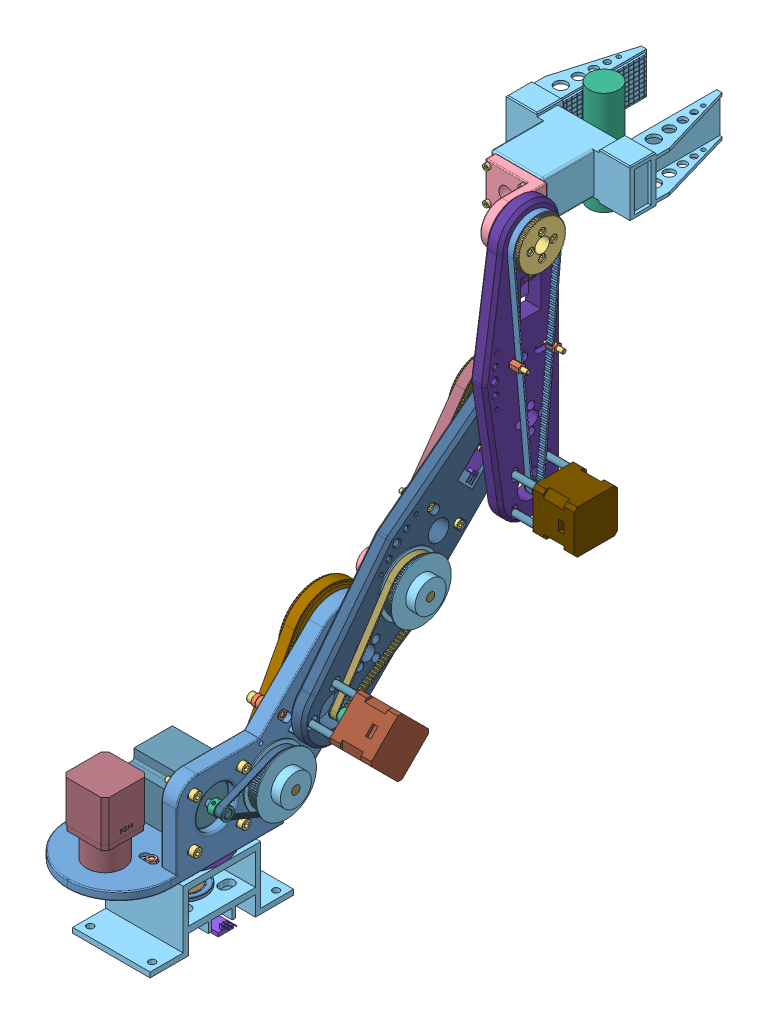
SolidWorks assembly R4 assem home axis, configuration Default. Lengths in mm. (continued)
Mates (geometry in assembly coordinates): (continued)
- Concentric8001: concentric anti-aligned: cylinder of PulleyHtd3m80Tbore8-2 through (18 150.2694 -118.5219) axis (1 0 0) radius 2.25; cylinder of socket head cap screw_iso0-144 through (-12.75 150.2694 -118.5219) axis (-1 0 0) radius 3.5
- Coincident7571: coincident anti-aligned: plane of PulleyHtd3m80Tbore8-2 through (23 150.2694 -118.5219) normal (-1 0 0); plane of socket head cap screw_iso0-144 through (23 153.7694 -118.5219) normal (1 0 0)
- Concentric8002: concentric aligned: cylinder of PulleyHtd3m80Tbore8-2 through (23 134.713 -118.5219) axis (-1 0 0) radius 3.6; cylinder of socket head cap screw_iso0-143 through (-12.75 134.713 -118.5219) axis (-1 0 0) radius 3.5
- Coincident7572: coincident anti-aligned: plane of PulleyHtd3m80Tbore8-2 through (23 134.713 -118.5219) normal (-1 0 0); plane of socket head cap screw_iso0-143 through (23 138.213 -118.5219) normal (1 0 0)
- Concentric8003: concentric anti-aligned: cylinder of PulleyHtd3m80Tbore8-2 through (18 134.713 -102.9655) axis (1 0 0) radius 2.25; cylinder of socket head cap screw_iso0-142 through (-12.75 134.713 -102.9655) axis (-1 0 0) radius 3.5
- Coincident7573: coincident anti-aligned: plane of PulleyHtd3m80Tbore8-2 through (23 134.713 -102.9655) normal (-1 0 0); plane of socket head cap screw_iso0-142 through (23 138.213 -102.9655) normal (1 0 0)
- Concentric8033: concentric anti-aligned: cylinder of MagneticSensorV2-2 through (50.9 117.7424 -93.066) axis (-1 0 0) radius 1.25; cylinder of socket head cap screw_iso1-80 through (83.15 117.7424 -93.066) axis (1 0 0) radius 1.9
- Coincident7610: coincident anti-aligned: plane of MagneticSensorV2-2 through (49.4 115.6211 -83.8737) normal (1 0 0); plane of socket head cap screw_iso1-80 through (49.4 117.0169 -91.31) normal (-1 0 0)
- Concentric8034: concentric anti-aligned: cylinder of MagneticSensorV2-2 through (50.9 124.8135 -85.995) axis (-1 0 0) radius 1.25; cylinder of socket head cap screw_iso1-81 through (83.15 124.8135 -85.995) axis (1 0 0) radius 1.9
- Coincident7611: coincident anti-aligned: plane of MagneticSensorV2-2 through (49.4 115.6211 -83.8737) normal (1 0 0); plane of socket head cap screw_iso1-81 through (49.4 124.088 -84.2389) normal (-1 0 0)
- Concentric8035: concentric aligned: cylinder of MagneticSensor-3 through (23.5 -42.0984 -5) axis (0 -1 0) radius 1.25; cylinder of socket head cap screw_iso-82 through (23.5 -83.3484 -5) axis (0 -1 0) radius 1.9
- Concentric8036: concentric aligned: cylinder of MagneticSensor-3 through (23.5 -42.0984 5) axis (0 -1 0) radius 1.25; cylinder of socket head cap screw_iso-83 through (23.5 -83.3484 5) axis (0 -1 0) radius 1.9
- Coincident7612: coincident anti-aligned: plane of MagneticSensor-3 through (31.5 -49.5984 0) normal (0 -1 0); plane of socket head cap screw_iso-83 through (21.6 -49.5984 5) normal (0 1 0)
- Concentric8037: concentric aligned: cylinder of base-1 through (23.5 -46.0984 -5) axis (0 1 0) radius 1.25; cylinder of hex nut style 1 gradeab_iso-23 through (23.5 -66.0359 -5) axis (0 1 0) radius 1
- Coincident7613: coincident anti-aligned: plane of base-1 through (31 -42.5984 13) normal (0 1 0); plane of hex nut style 1 gradeab_iso-23 through (23.5 -42.5984 -7.3094) normal (0 -1 0)
- Concentric8038: concentric aligned: cylinder of base-1 through (23.5 -46.0984 5) axis (0 1 0) radius 1.25; cylinder of hex nut style 1 gradeab_iso-24 through (23.5 -66.0359 5) axis (0 1 0) radius 1
- Coincident7614: coincident anti-aligned: plane of base-1 through (31 -42.5984 13) normal (0 1 0); plane of hex nut style 1 gradeab_iso-24 through (23.5 -42.5984 2.6906) normal (0 -1 0)
- Concentric8039: concentric anti-aligned: cylinder of arm1-1 through (35 117.7424 -93.066) axis (1 0 0) radius 1.25; cylinder of hex nut style 1 gradeab_isoV1-25 through (62.4375 117.7424 -93.066) axis (-1 0 0) radius 1
- Coincident7615: coincident anti-aligned: plane of arm1-1 through (39 22.25 32) normal (-1 0 0); plane of hex nut style 1 gradeab_isoV1-25 through (39 120.0519 -93.066) normal (1 0 0)
- Concentric8040: concentric anti-aligned: cylinder of arm1-1 through (35 124.8135 -85.995) axis (1 0 0) radius 1.25; cylinder of hex nut style 1 gradeab_isoV1-26 through (62.4375 124.8135 -85.995) axis (-1 0 0) radius 1
- Coincident7616: coincident anti-aligned: plane of arm1-1 through (39 22.25 32) normal (-1 0 0); plane of hex nut style 1 gradeab_isoV1-26 through (39 127.1229 -85.995) normal (1 0 0)
- Concentric8058: concentric aligned: cylinder of Nema23_57x57x56-2 through (-12 91.32 40.6675) axis (1 0 0) radius 2.75; cylinder of socket head cap screw_iso1-96 through (86.75 91.32 40.6675) axis (1 0 0) radius 2.5
- Coincident7633: coincident anti-aligned: plane of arm1-1 through (50 30.25 -48) normal (1 0 0); plane of socket head cap screw_iso1-96 through (50 92.9429 36.7395) normal (-1 0 0)
- Coincident76341: coincident anti-aligned: plane of arm1-1 through (50 30.25 -48) normal (1 0 0); plane of socket head cap screw_iso1-98 through (50 45.8029 -10.4005) normal (-1 0 0)
- Coincident76351: coincident anti-aligned: plane of arm1-1 through (50 30.25 -48) normal (1 0 0); plane of socket head cap screw_iso1-99 through (50 45.8029 36.7395) normal (-1 0 0)
- Concentric8059: concentric aligned: cylinder of Nema23_57x57x56-2 through (-12 44.18 40.6675) axis (1 0 0) radius 2.75; cylinder of socket head cap screw_iso1-99 through (86.75 44.18 40.6675) axis (1 0 0) radius 4.25
- Concentric8060: concentric aligned: cylinder of Nema23_57x57x56-2 through (-12 44.18 -6.4725) axis (1 0 0) radius 2.75; circle of socket head cap screw_iso-98
- Concentric8061: concentric aligned: cylinder of Nema23_57x57x56-2 through (-12 91.32 -6.4725) axis (1 0 0) radius 2.75; cylinder of socket head cap screw_iso1-97 through (86.75 91.32 -6.4725) axis (1 0 0) radius 4.25
- Coincident7636: coincident aligned: plane of arm1-1 through (50 30.25 -48) normal (1 0 0); circle of socket head cap screw_iso-97
- Concentric8066: concentric aligned: cylinder of arm1-1 through (9.8995 30.25 85.4995) axis (0 -1 0) radius 1.65; cylinder of socket head cap screw_iso1-104 through (9.8995 -12.5 85.4995) axis (0 -1 0) radius 2.75
- Coincident7641: coincident anti-aligned: plane of arm1-1 through (0 22.25 32) normal (0 -1 0); plane of socket head cap screw_iso1-104 through (7.1495 22.25 85.4995) normal (0 1 0)
- Concentric80671: concentric aligned: cylinder of arm1-1 through (9.8995 30.25 65.7005) axis (0 -1 0) radius 1.65; cylinder of socket head cap screw_iso1-105 through (9.8995 -12.5 65.7005) axis (0 -1 0) radius 2.75
- Coincident76421: coincident anti-aligned: plane of arm1-1 through (0 22.25 32) normal (0 -1 0); plane of socket head cap screw_iso1-105 through (7.1495 22.25 65.7005) normal (0 1 0)
- Concentric8068: concentric aligned: cylinder of arm1-1 through (-9.8995 30.25 85.4995) axis (0 -1 0) radius 1.65; cylinder of socket head cap screw_iso1-106 through (-9.8995 -12.5 85.4995) axis (0 -1 0) radius 2.75
- Coincident7643: coincident anti-aligned: plane of arm1-1 through (0 22.25 32) normal (0 -1 0); plane of socket head cap screw_iso1-106 through (-12.6495 22.25 85.4995) normal (0 1 0)
- Concentric8069: concentric aligned: cylinder of arm1-1 through (-9.8995 30.25 65.7005) axis (0 -1 0) radius 1.65; cylinder of socket head cap screw_iso1-107 through (-9.8995 -12.5 65.7005) axis (0 -1 0) radius 2.75
- Coincident7644: coincident anti-aligned: plane of arm1-1 through (0 22.25 32) normal (0 -1 0); plane of socket head cap screw_iso1-107 through (-12.6495 22.25 65.7005) normal (0 1 0)
- Coincident76428: coincident aligned: plane of MagneticSensor-3 through (31.5 -49.5984 0) normal (0 -1 0); circle of socket head cap screw_iso-82
- Concentric80674: concentric anti-aligned: cylinder of socket head cap screw_iso1-96 through (86.75 91.32 40.6675) axis (1 0 0) radius 2.5; cylinder of hex nut style 1 gradeab_isoV1-35 through (55.3375 91.32 40.6675) axis (-1 0 0) radius 2.5
- Coincident76429: coincident anti-aligned: plane of Nema23_57x57x56-2 through (35 67.75 17.0975) normal (-1 0 0); plane of hex nut style 1 gradeab_isoV1-35 through (35 91.32 32.6675) normal (1 0 0)
- Concentric80675: concentric anti-aligned: cylinder of Nema23_57x57x56-2 through (-12 91.32 -6.4725) axis (1 0 0) radius 2.75; cylinder of hex nut style 1 gradeab_isoV1-36 through (55.3375 91.32 -6.4725) axis (-1 0 0) radius 2.5
- Coincident76430: coincident anti-aligned: plane of Nema23_57x57x56-2 through (35 67.75 17.0975) normal (-1 0 0); plane of hex nut style 1 gradeab_isoV1-36 through (35 91.32 -14.4725) normal (1 0 0)
- Concentric80676: concentric anti-aligned: cylinder of Nema23_57x57x56-2 through (-12 44.18 -6.4725) axis (1 0 0) radius 2.75; cylinder of hex nut style 1 gradeab_isoV1-37 through (55.3375 44.18 -6.4725) axis (-1 0 0) radius 2.5
- Coincident76431: coincident anti-aligned: plane of Nema23_57x57x56-2 through (35 67.75 17.0975) normal (-1 0 0); plane of hex nut style 1 gradeab_isoV1-37 through (35 44.18 -14.4725) normal (1 0 0)
- Concentric80677: concentric aligned: cylinder of socket head cap screw_iso1-99 through (86.75 44.18 40.6675) axis (1 0 0) radius 2.5; cylinder of hex nut style 1 gradeab_isoV1-38 through (15.3591 44.18 40.6675) axis (1 0 0) radius 2.5
- Concentric80678: concentric anti-aligned: cylinder of arm2-1 through (68 280.4336 -248.6861) axis (-1 0 0) radius 21; cylinder of bearing6806 30x42x7-5 through (68 280.4336 -248.6861) axis (1 0 0) radius 21
- Coincident76432: coincident anti-aligned: plane of arm2-1 through (61 280.4336 -248.6861) normal (1 0 0); plane of bearing6806 30x42x7-5 through (61 301.0275 -250.2074) normal (-1 0 0)
- Coincident76433: coincident anti-aligned: plane of arm2-1 through (60 280.4336 -248.6861) normal (-1 0 0); plane of bearing6806 30x42x7-6 through (60 299.5086 -240.7761) normal (1 0 0)
- Concentric80679: concentric aligned: cylinder of arm2-1 through (68 280.4336 -248.6861) axis (-1 0 0) radius 21; cylinder of bearing6806 30x42x7-6 through (53 280.4336 -248.6861) axis (-1 0 0) radius 21
- Coincident76434: coincident anti-aligned: plane of arm2-1 through (61 181.3255 -149.578) normal (1 0 0); plane of bearing608 8x22x7-3 through (61 181.3255 -149.578) normal (-1 0 0)
- Concentric80680: concentric anti-aligned: cylinder of arm2-1 through (68 181.3255 -149.578) axis (-1 0 0) radius 11; cylinder of bearing608 8x22x7-3 through (61 181.3255 -149.578) axis (1 0 0) radius 11
- Concentric80681: concentric anti-aligned: cylinder of arm2-1 through (68 181.3255 -149.578) axis (-1 0 0) radius 11; cylinder of bearing608 8x22x7-4 through (53 181.3255 -149.578) axis (1 0 0) radius 11
- Coincident76436: coincident anti-aligned: plane of arm2-1 through (60 181.3255 -149.578) normal (-1 0 0); plane of bearing608 8x22x7-4 through (60 181.3255 -149.578) normal (1 0 0)
- Concentric80682: concentric anti-aligned: cylinder of arm2-1 through (68 110.6714 -78.9239) axis (-1 0 0) radius 15; cylinder of nema17L48arm2-1 through (68 110.6714 -78.9239) axis (1 0 0) radius 2.5
- Coincident76437: coincident anti-aligned: plane of arm2-1 through (68 280.4336 -248.6861) normal (1 0 0); plane of nema17L48arm2-1 through (68 110.6714 -78.9239) normal (-1 0 0)
- Parallel3: parallel aligned: plane of arm2-1 through (68 88.7199 -99.3726) normal (0 -0.707107 -0.707107); plane of nema17L48arm2-1 through (101 106.4287 -104.3798) normal (0 -0.707107 -0.707107)
- Concentric80684: concentric anti-aligned: cylinder of nema17L48arm2-1 through (68 110.6714 -78.9239) axis (1 0 0) radius 2.5; cylinder of pulley2GT16Tbore6.35-2 through (82 110.6714 -78.9239) axis (-1 0 0) radius 4
- Coincident76439: coincident anti-aligned: plane of arm2-1 through (68 280.4336 -248.6861) normal (1 0 0); plane of pulley2GT16Tbore6.35-2 through (68 110.6714 -78.9239) normal (-1 0 0)
- Coincident76440: coincident anti-aligned: plane of arm2-1 through (68 280.4336 -248.6861) normal (1 0 0); plane of pulley2GT80T-2 through (68 181.3255 -149.578) normal (-1 0 0)
- Concentric80686: concentric aligned: cylinder of bearing608 8x22x7-3 through (61 181.3255 -149.578) axis (1 0 0) radius 4; cylinder of pulley2GT80T-2 through (68 181.3255 -149.578) axis (1 0 0) radius 4
- Concentric80687: concentric aligned: cylinder of pulley2GT16Tbore6.35-2 through (82 110.6714 -78.9239) axis (-1 0 0) radius 6.1; cylinder of belt2GTarm2-1 through (75 110.6714 -78.9239) axis (-1 0 0) radius 5.723
- Concentric80688: concentric anti-aligned: cylinder of pulley2GT80T-2 through (68 181.3255 -149.578) axis (1 0 0) radius 4; cylinder of belt2GTarm2-1 through (75 181.3255 -149.578) axis (-1 0 0) radius 26.0948
- Coincident76441: coincident anti-aligned: plane of pulley2GT16Tbore6.35-2 through (69 110.6714 -78.9239) normal (1 0 0); plane of belt2GTarm2-1 through (69 181.3255 -149.578) normal (-1 0 0)
- Concentric80689: concentric anti-aligned: cylinder of pulley2GT80T-2 through (68 181.3255 -149.578) axis (1 0 0) radius 4; cylinder of shaft8x70-2 through (90 181.3255 -149.578) axis (-1 0 0) radius 4
- Coincident76442: coincident aligned: plane of pulley2GT80T-2 through (90 181.3255 -149.578) normal (1 0 0); plane of shaft8x70-2 through (90 181.3255 -149.578) normal (1 0 0)
- Concentric80690: concentric anti-aligned: cylinder of shaft8x70-2 through (90 181.3255 -149.578) axis (-1 0 0) radius 4; cylinder of Pulleyhtd3m20Tbore8-2 through (29 181.3255 -149.578) axis (1 0 0) radius 4
- Coincident76443: coincident anti-aligned: plane of arm2-1 through (53 280.4336 -248.6861) normal (-1 0 0); plane of Pulleyhtd3m20Tbore8-2 through (53 181.3255 -149.578) normal (1 0 0)
- Concentric80691: concentric aligned: cylinder of bearing6806 30x42x7-5 through (68 280.4336 -248.6861) axis (1 0 0) radius 14.9995; cylinder of PulleyHtd3m80Tbore8arm2-1 through (38 280.4336 -248.6861) axis (1 0 0) radius 7
- Coincident76444: coincident anti-aligned: plane of arm2-1 through (53 280.4336 -248.6861) normal (-1 0 0); plane of PulleyHtd3m80Tbore8arm2-1 through (53 280.4336 -248.6861) normal (1 0 0)
- Concentric80692: concentric anti-aligned: cylinder of Pulleyhtd3m20Tbore8-2 through (29 181.3255 -149.578) axis (1 0 0) radius 11; cylinder of beltHTD3marm2-1 through (52 181.3255 -149.578) axis (-1 0 0) radius 10.3983
- Concentric80693: concentric anti-aligned: cylinder of beltHTD3marm2-1 through (52 280.4336 -248.6861) axis (-1 0 0) radius 33.7941; cylinder of PulleyHtd3m80Tbore8arm2-1 through (38 280.4336 -248.6861) axis (1 0 0) radius 7
- Coincident76445: coincident anti-aligned: plane of Pulleyhtd3m20Tbore8-2 through (52 181.3255 -149.578) normal (-1 0 0); plane of beltHTD3marm2-1 through (52 280.4336 -248.6861) normal (1 0 0)
- Concentric80697: concentric anti-aligned: cylinder of PulleyHtd3m80Tbore8-2 through (18 142.4912 -110.7437) axis (1 0 0) radius 7; cylinder of arm2-1 through (68 142.4912 -110.7437) axis (-1 0 0) radius 7
- Concentric80698: concentric aligned: cylinder of bearingCover-1 through (53 134.713 -102.9655) axis (-1 0 0) radius 2.25; cylinder of arm2-1 through (68 134.713 -102.9655) axis (-1 0 0) radius 2.25
- Coincident76451: coincident anti-aligned: plane of bearingCover-1 through (53 142.4912 -110.7437) normal (1 0 0); plane of arm2-1 through (53 280.4336 -248.6861) normal (-1 0 0)
- Concentric80700: concentric anti-aligned: cylinder of arm3-1 through (88 431.1836 -248.6861) axis (-1 0 0) radius 21; cylinder of bearing6806 30x42x7-7 through (88 431.1836 -248.6861) axis (1 0 0) radius 21
- Coincident76452: coincident anti-aligned: plane of arm3-1 through (81 431.1836 -248.6861) normal (1 0 0); plane of bearing6806 30x42x7-7 through (81 451.8336 -248.6861) normal (-1 0 0)
- Coincident76453: coincident anti-aligned: plane of arm3-1 through (80 431.1836 -248.6861) normal (-1 0 0); plane of bearing6806 30x42x7-8 through (80 451.8336 -248.6861) normal (1 0 0)
- Concentric80701: concentric anti-aligned: cylinder of arm3-1 through (88 431.1836 -248.6861) axis (-1 0 0) radius 21; cylinder of bearing6806 30x42x7-8 through (80 431.1836 -248.6861) axis (1 0 0) radius 21
- Concentric80702: concentric anti-aligned: cylinder of arm3-1 through (88 225.4336 -248.6861) axis (-1 0 0) radius 13; cylinder of nema17L48arm3-1 through (88 225.4336 -248.6861) axis (1 0 0) radius 2.5
- Coincident76454: coincident anti-aligned: plane of arm3-1 through (88 431.1836 -248.6861) normal (1 0 0); plane of nema17L48arm3-1 through (88 225.4336 -248.6861) normal (-1 0 0)
- Parallel5: parallel aligned: plane of arm3-1 through (88 225.4336 -278.6861) normal (0 0 -1); plane of nema17L48arm3-1 through (121 240.4336 -269.6861) normal (0 0 -1)
- Concentric80704: concentric anti-aligned: cylinder of nema17L48arm3-1 through (88 225.4336 -248.6861) axis (1 0 0) radius 2.5; cylinder of pulley2GT16Tbore6.35-3 through (102 225.4336 -248.6861) axis (-1 0 0) radius 4
- Coincident76457: coincident anti-aligned: plane of arm3-1 through (88 431.1836 -248.6861) normal (1 0 0); plane of pulley2GT16Tbore6.35-3 through (88 225.4336 -248.6861) normal (-1 0 0)
- Concentric80705: concentric anti-aligned: cylinder of bearing6806 30x42x7-8 through (80 431.1836 -248.6861) axis (1 0 0) radius 14.9995; cylinder of pulley2GT60T-1 through (99 431.1836 -248.6861) axis (-1 0 0) radius 7
- Coincident76458: coincident anti-aligned: plane of arm3-1 through (88 431.1836 -248.6861) normal (1 0 0); plane of pulley2GT60T-1 through (88 431.1836 -248.6861) normal (-1 0 0)
- Concentric80706: concentric aligned: cylinder of pulley2GT16Tbore6.35-3 through (102 225.4336 -248.6861) axis (-1 0 0) radius 6.1; cylinder of belt2GTarm3-1 through (95 225.4336 -248.6861) axis (-1 0 0) radius 5.942
- Concentric80707: concentric aligned: cylinder of pulley2GT60T-1 through (99 431.1836 -248.6861) axis (-1 0 0) radius 7; cylinder of belt2GTarm3-1 through (95 431.1836 -248.6861) axis (-1 0 0) radius 23.7673
- Coincident76459: coincident anti-aligned: plane of pulley2GT16Tbore6.35-3 through (89 225.4336 -248.6861) normal (1 0 0); plane of belt2GTarm3-1 through (89 431.1836 -248.6861) normal (-1 0 0)
- Coincident76460: coincident anti-aligned: plane of arm3-1 through (78 225.4336 -248.6861) normal (-1 0 0); plane of MagneticSensor-4 through (78 386.1836 -248.6861) normal (1 0 0)
- Concentric80708: concentric anti-aligned: cylinder of arm3-1 through (83 394.1836 -243.6861) axis (-1 0 0) radius 1.25; cylinder of MagneticSensor-4 through (70.5 394.1836 -243.6861) axis (1 0 0) radius 1.25
- Parallel6: parallel aligned: plane of arm3-1 through (88 225.4336 -278.6861) normal (0 0 -1); plane of MagneticSensor-4 through (74.5 396.1836 -256.1861) normal (0 0 -1)
- Coincident76462: coincident anti-aligned: plane of PulleyHtd3m80Tbore8arm2-1 through (70 280.4336 -248.6861) normal (1 0 0); plane of bearingCover-2 through (70 280.4336 -248.6861) normal (-1 0 0)
- Concentric80710: concentric aligned: cylinder of PulleyHtd3m80Tbore8arm2-1 through (38 280.4336 -248.6861) axis (1 0 0) radius 7; cylinder of bearingCover-2 through (70 280.4336 -248.6861) axis (1 0 0) radius 7
- Concentric80711: concentric aligned: cylinder of PulleyHtd3m80Tbore8arm2-1 through (38 291.4336 -248.6861) axis (1 0 0) radius 2.25; cylinder of bearingCover-2 through (70 291.4336 -248.6861) axis (1 0 0) radius 2.25
- Concentric80712: concentric anti-aligned: cylinder of PulleyHtd3m80Tbore8arm2-1 through (38 280.4336 -248.6861) axis (1 0 0) radius 7; cylinder of arm3-1 through (88 280.4336 -248.6861) axis (-1 0 0) radius 7
- Concentric80713: concentric anti-aligned: cylinder of arm3-1 through (88 291.4336 -248.6861) axis (-1 0 0) radius 2.25; cylinder of bearingCover-2 through (70 291.4336 -248.6861) axis (1 0 0) radius 2.25
- Coincident76463: coincident anti-aligned: plane of arm3-1 through (73 431.1836 -248.6861) normal (-1 0 0); plane of bearingCover-2 through (73 280.4336 -248.6861) normal (1 0 0)
- Coincident76464: coincident anti-aligned: plane of pulley2GT60T-1 through (72 431.1836 -248.6861) normal (-1 0 0); plane of bearingCover-3 through (72 431.1836 -248.6861) normal (1 0 0)
- Concentric80715: concentric anti-aligned: cylinder of pulley2GT60T-1 through (99 431.1836 -248.6861) axis (-1 0 0) radius 7; cylinder of bearingCover-3 through (69 431.1836 -248.6861) axis (1 0 0) radius 7
- Concentric80716: concentric anti-aligned: cylinder of pulley2GT60T-1 through (99 431.1836 -259.6861) axis (-1 0 0) radius 2.25; cylinder of bearingCover-3 through (69 431.1836 -259.6861) axis (1 0 0) radius 2.25
- Concentric80717: concentric anti-aligned: cylinder of pulley2GT60T-1 through (99 431.1836 -248.6861) axis (-1 0 0) radius 7; cylinder of gripper holder-1 through (59 431.1836 -248.6861) axis (1 0 0) radius 7
- Concentric80718: concentric aligned: cylinder of gripper holder-1 through (59 431.1836 -259.6861) axis (1 0 0) radius 2.25; cylinder of bearingCover-3 through (69 431.1836 -259.6861) axis (1 0 0) radius 2.25
- Coincident76465: coincident anti-aligned: plane of gripper holder-1 through (69 431.1836 -248.6861) normal (1 0 0); plane of bearingCover-3 through (69 431.1836 -248.6861) normal (-1 0 0)
- Concentric80719: concentric aligned: cylinder of gripper holder-1 through (39 431.1836 -283.6861) axis (0 0 1) radius 7; cylinder of Part1g-1 through (39.0001 431.1835 -285.6861) axis (0 0 1) radius 5
- Concentric80720: concentric aligned: cylinder of gripper holder-1 through (21.78 446.6859 -283.6861) axis (0 0 1) radius 1.55; cylinder of Part1g-1 through (21.78 446.6859 -285.6861) axis (0 0 1) radius 1.55
- Coincident76466: coincident anti-aligned: plane of gripper holder-1 through (69 451.1836 -283.6861) normal (0 0 -1); plane of Part1g-1 through (39.0001 431.1835 -283.6861) normal (0 0 1)
- Concentric80721: concentric aligned: cylinder of nema17L48arm2-1 through (96 110.6714 -56.2965) axis (-1 0 0) radius 1.5; cylinder of cover nuts-1 through (91 110.6714 -56.2965) axis (-1 0 0) radius 1.5
- Coincident76470: coincident anti-aligned: plane of nema17L48arm2-1 through (91 140.3699 -78.9239) normal (-1 0 0); plane of cover nuts-1 through (91 110.6714 -56.2965) normal (1 0 0)
- Concentric80722: concentric aligned: cylinder of nema17L48arm2-1 through (96 133.2988 -78.9239) axis (-1 0 0) radius 1.5; cylinder of cover nuts-2 through (91 133.2988 -78.9239) axis (-1 0 0) radius 1.5
- Coincident76471: coincident anti-aligned: plane of nema17L48arm2-1 through (91 140.3699 -78.9239) normal (-1 0 0); plane of cover nuts-2 through (91 133.2988 -78.9239) normal (1 0 0)
- Concentric80723: concentric aligned: cylinder of nema17L48arm2-1 through (96 88.044 -78.9239) axis (-1 0 0) radius 1.5; cylinder of cover nuts-3 through (91 88.044 -78.9239) axis (-1 0 0) radius 1.5
- Coincident76472: coincident anti-aligned: plane of nema17L48arm2-1 through (91 140.3699 -78.9239) normal (-1 0 0); plane of cover nuts-3 through (91 88.044 -78.9239) normal (1 0 0)
- Concentric80724: concentric anti-aligned: cylinder of nema17L48arm2-1 through (96 110.6714 -101.5513) axis (-1 0 0) radius 1.5; cylinder of cover nuts-4 through (68 110.6714 -101.5513) axis (1 0 0) radius 1.5
- Coincident76473: coincident anti-aligned: plane of nema17L48arm2-1 through (91 140.3699 -78.9239) normal (-1 0 0); plane of cover nuts-4 through (91 110.6714 -101.5513) normal (1 0 0)
- Concentric80725: concentric aligned: cylinder of nema17L48arm3-1 through (116 209.4336 -232.6861) axis (-1 0 0) radius 1.5; cylinder of cover nuts-5 through (111 209.4336 -232.6861) axis (-1 0 0) radius 1.5
- Coincident76474: coincident anti-aligned: plane of nema17L48arm3-1 through (111 246.4336 -227.6861) normal (-1 0 0); plane of cover nuts-5 through (111 209.4336 -232.6861) normal (1 0 0)
- Concentric80726: concentric aligned: cylinder of nema17L48arm3-1 through (116 241.4336 -232.6861) axis (-1 0 0) radius 1.5; cylinder of cover nuts-6 through (111 241.4336 -232.6861) axis (-1 0 0) radius 1.5
- Coincident76475: coincident anti-aligned: plane of nema17L48arm3-1 through (111 246.4336 -227.6861) normal (-1 0 0); plane of cover nuts-6 through (111 241.4336 -232.6861) normal (1 0 0)
- Concentric80727: concentric aligned: cylinder of nema17L48arm3-1 through (116 209.4336 -264.6861) axis (-1 0 0) radius 1.5; cylinder of cover nuts-7 through (111 209.4336 -264.6861) axis (-1 0 0) radius 1.5
- Coincident76476: coincident anti-aligned: plane of nema17L48arm3-1 through (111 246.4336 -227.6861) normal (-1 0 0); plane of cover nuts-7 through (111 209.4336 -264.6861) normal (1 0 0)
- Concentric80728: concentric aligned: cylinder of nema17L48arm3-1 through (116 241.4336 -264.6861) axis (-1 0 0) radius 1.5; cylinder of cover nuts-8 through (111 241.4336 -264.6861) axis (-1 0 0) radius 1.5
- Coincident76477: coincident anti-aligned: plane of nema17L48arm3-1 through (111 246.4336 -227.6861) normal (-1 0 0); plane of cover nuts-8 through (111 241.4336 -264.6861) normal (1 0 0)
- Concentric80740: concentric anti-aligned: cylinder of PulleyHtd3m80Tbore8arm2-1 through (38 269.4336 -248.6861) axis (1 0 0) radius 2.25; cylinder of socket head cap screw_iso0-193 through (7.25 269.4336 -248.6861) axis (-1 0 0) radius 3.5
- Coincident76489: coincident anti-aligned: plane of PulleyHtd3m80Tbore8arm2-1 through (43 269.4336 -248.6861) normal (-1 0 0); plane of socket head cap screw_iso0-193 through (43 272.9336 -248.6861) normal (1 0 0)
- Concentric80741: concentric anti-aligned: cylinder of PulleyHtd3m80Tbore8arm2-1 through (38 291.4336 -248.6861) axis (1 0 0) radius 2.25; cylinder of socket head cap screw_iso0-194 through (7.25 291.4336 -248.6861) axis (-1 0 0) radius 3.5
- Coincident76490: coincident anti-aligned: plane of PulleyHtd3m80Tbore8arm2-1 through (43 291.4336 -248.6861) normal (-1 0 0); plane of socket head cap screw_iso0-194 through (43 294.9336 -248.6861) normal (1 0 0)
- Concentric80742: concentric anti-aligned: cylinder of PulleyHtd3m80Tbore8arm2-1 through (38 280.4336 -237.6861) axis (1 0 0) radius 2.25; cylinder of socket head cap screw_iso0-195 through (7.25 280.4336 -237.6861) axis (-1 0 0) radius 3.5
- Coincident76491: coincident anti-aligned: plane of PulleyHtd3m80Tbore8arm2-1 through (43 280.4336 -237.6861) normal (-1 0 0); plane of socket head cap screw_iso0-195 through (43 283.9336 -237.6861) normal (1 0 0)
- Concentric80743: concentric anti-aligned: cylinder of PulleyHtd3m80Tbore8arm2-1 through (38 280.4336 -259.6861) axis (1 0 0) radius 2.25; cylinder of socket head cap screw_iso0-196 through (7.25 280.4336 -259.6861) axis (-1 0 0) radius 3.5
- Coincident76492: coincident anti-aligned: plane of PulleyHtd3m80Tbore8arm2-1 through (43 280.4336 -259.6861) normal (-1 0 0); plane of socket head cap screw_iso0-196 through (43 283.9336 -259.6861) normal (1 0 0)
- Concentric80746: concentric aligned: cylinder of arm2-1 through (68 233.411 -172.6721) axis (-1 0 0) radius 2.5; cylinder of hex thin nut chamfered gradeab_iso-2 through (75.8375 233.411 -172.6721) axis (-1 0 0) radius 2
- Coincident76495: coincident anti-aligned: plane of arm2-1 through (53 280.4336 -248.6861) normal (-1 0 0); plane of hex thin nut chamfered gradeab_iso-2 through (53 237.4524 -172.6721) normal (1 0 0)
- Concentric80747: concentric anti-aligned: cone of hex thin nut chamfered gradeab_iso-2 through (51.0696 233.411 -172.6721) axis (1 0 0); cylinder of hex thin nut chamfered gradeab_iso-3 through (73.6375 233.411 -172.6721) axis (-1 0 0) radius 2
- Coincident76496: coincident anti-aligned: plane of hex thin nut chamfered gradeab_iso-2 through (50.8 237.4524 -172.6721) normal (-1 0 0); plane of hex thin nut chamfered gradeab_iso-3 through (50.8 237.4524 -172.6721) normal (1 0 0)
- Concentric80748: concentric anti-aligned: cylinder of hex thin nut chamfered gradeab_iso-3 through (48.8696 233.411 -172.6721) axis (1 0 0) radius 959.9311; cylinder of hex thin nut chamfered gradeab_iso-4 through (71.4375 233.411 -172.6721) axis (-1 0 0) radius 2
- Coincident76497: coincident anti-aligned: plane of hex thin nut chamfered gradeab_iso-3 through (48.6 237.4524 -172.6721) normal (-1 0 0); plane of hex thin nut chamfered gradeab_iso-4 through (48.6 237.4524 -172.6721) normal (1 0 0)
- Concentric80749: concentric anti-aligned: cylinder of hex thin nut chamfered gradeab_iso-4 through (46.6696 233.411 -172.6721) axis (1 0 0) radius 959.9311; cylinder of hex thin nut chamfered gradeab_iso-5 through (69.2375 233.411 -172.6721) axis (-1 0 0) radius 2
- Coincident76498: coincident anti-aligned: plane of hex thin nut chamfered gradeab_iso-4 through (46.4 237.4524 -172.6721) normal (-1 0 0); plane of hex thin nut chamfered gradeab_iso-5 through (46.4 237.4524 -172.6721) normal (1 0 0)
- Concentric80750: concentric anti-aligned: cylinder of hex thin nut chamfered gradeab_iso-5 through (44.4696 233.411 -172.6721) axis (1 0 0) radius 959.9311; cylinder of hex thin nut chamfered gradeab_iso-6 through (67.0375 233.411 -172.6721) axis (-1 0 0) radius 2
- Coincident76499: coincident anti-aligned: plane of hex thin nut chamfered gradeab_iso-5 through (44.2 237.4524 -172.6721) normal (-1 0 0); plane of hex thin nut chamfered gradeab_iso-6 through (44.2 237.4524 -172.6721) normal (1 0 0)
- Concentric80751: concentric aligned: cylinder of arm2-1 through (68 204.4196 -201.6635) axis (-1 0 0) radius 2.5; cylinder of hex thin nut chamfered gradeab_iso-7 through (75.8375 204.4196 -201.6635) axis (-1 0 0) radius 2
- Coincident76500: coincident anti-aligned: plane of arm2-1 through (53 280.4336 -248.6861) normal (-1 0 0); plane of hex thin nut chamfered gradeab_iso-7 through (53 208.4611 -201.6635) normal (1 0 0)
- Concentric80752: concentric anti-aligned: cylinder of hex thin nut chamfered gradeab_iso-7 through (51.0696 204.4196 -201.6635) axis (1 0 0) radius 959.9311; cylinder of hex thin nut chamfered gradeab_iso-8 through (73.6375 204.4196 -201.6635) axis (-1 0 0) radius 2
- Coincident76501: coincident anti-aligned: plane of hex thin nut chamfered gradeab_iso-7 through (50.8 208.4611 -201.6635) normal (-1 0 0); plane of hex thin nut chamfered gradeab_iso-8 through (50.8 208.4611 -201.6635) normal (1 0 0)
- Concentric80753: concentric anti-aligned: cylinder of hex thin nut chamfered gradeab_iso-8 through (48.8696 204.4196 -201.6635) axis (1 0 0) radius 959.9311; cylinder of hex thin nut chamfered gradeab_iso-9 through (71.4375 204.4196 -201.6635) axis (-1 0 0) radius 2
- Coincident76502: coincident anti-aligned: plane of hex thin nut chamfered gradeab_iso-8 through (48.6 208.4611 -201.6635) normal (-1 0 0); plane of hex thin nut chamfered gradeab_iso-9 through (48.6 208.4611 -201.6635) normal (1 0 0)
- Concentric80754: concentric anti-aligned: cylinder of hex thin nut chamfered gradeab_iso-9 through (46.6696 204.4196 -201.6635) axis (1 0 0) radius 959.9311; cylinder of hex thin nut chamfered gradeab_iso-10 through (69.2375 204.4196 -201.6635) axis (-1 0 0) radius 2
- Coincident76503: coincident anti-aligned: plane of hex thin nut chamfered gradeab_iso-9 through (46.4 208.4611 -201.6635) normal (-1 0 0); plane of hex thin nut chamfered gradeab_iso-10 through (46.4 208.4611 -201.6635) normal (1 0 0)
- Concentric80755: concentric anti-aligned: cylinder of hex thin nut chamfered gradeab_iso-10 through (44.4696 204.4196 -201.6635) axis (1 0 0) radius 959.9311; cylinder of hex thin nut chamfered gradeab_iso-11 through (67.0375 204.4196 -201.6635) axis (-1 0 0) radius 2
- Coincident76504: coincident anti-aligned: plane of hex thin nut chamfered gradeab_iso-10 through (44.2 208.4611 -201.6635) normal (-1 0 0); plane of hex thin nut chamfered gradeab_iso-11 through (44.2 208.4611 -201.6635) normal (1 0 0)
- Concentric80756: concentric anti-aligned: cylinder of arm2-1 through (63 259.2204 -220.4018) axis (-1 0 0) radius 1.25; cylinder of hex thin nut chamfered gradeab_iso-12 through (39.1625 259.2204 -220.4018) axis (1 0 0) radius 1
- Coincident76505: coincident anti-aligned: plane of arm2-1 through (63 110.6714 -78.9239) normal (1 0 0); plane of hex thin nut chamfered gradeab_iso-12 through (63 261.5298 -220.4018) normal (-1 0 0)
- Concentric80757: concentric anti-aligned: cylinder of arm2-1 through (63 252.1493 -227.4729) axis (-1 0 0) radius 1.25; cylinder of hex thin nut chamfered gradeab_iso-13 through (39.1625 252.1493 -227.4729) axis (1 0 0) radius 1
- Coincident76506: coincident anti-aligned: plane of arm2-1 through (63 110.6714 -78.9239) normal (1 0 0); plane of hex thin nut chamfered gradeab_iso-13 through (63 254.4587 -227.4729) normal (-1 0 0)
- Concentric80762: concentric anti-aligned: cylinder of MagneticSensor-4 through (70.5 394.1836 -243.6861) axis (1 0 0) radius 1.25; cylinder of socket head cap screw_iso0-197 through (40.75 394.1836 -243.6861) axis (-1 0 0) radius 1.9
- Coincident76511: coincident anti-aligned: plane of MagneticSensor-4 through (74.5 386.1836 -248.6861) normal (-1 0 0); plane of socket head cap screw_iso0-197 through (74.5 396.0836 -243.6861) normal (1 0 0)
- Concentric80763: concentric anti-aligned: cylinder of MagneticSensor-4 through (70.5 394.1836 -253.6861) axis (1 0 0) radius 1.25; cylinder of socket head cap screw_iso0-198 through (40.75 394.1836 -253.6861) axis (-1 0 0) radius 1.9
- Coincident76512: coincident anti-aligned: plane of MagneticSensor-4 through (74.5 386.1836 -248.6861) normal (-1 0 0); plane of socket head cap screw_iso0-198 through (74.5 396.0836 -253.6861) normal (1 0 0)
- Concentric80767: concentric anti-aligned: cylinder of arm3-1 through (83 394.1836 -243.6861) axis (-1 0 0) radius 1.25; cylinder of hex thin nut gradeb_iso00-2 through (59.1625 394.1836 -243.6861) axis (1 0 0) radius 1
- Coincident76516: coincident anti-aligned: plane of arm3-1 through (83 225.4336 -248.6861) normal (1 0 0); plane of hex thin nut gradeb_iso00-2 through (83 396.493 -243.6861) normal (-1 0 0)
- Concentric80768: concentric anti-aligned: cylinder of arm3-1 through (83 394.1836 -253.6861) axis (-1 0 0) radius 1.25; cylinder of hex thin nut gradeb_iso00-3 through (59.1625 394.1836 -253.6861) axis (1 0 0) radius 1
- Coincident76517: coincident anti-aligned: plane of arm3-1 through (83 225.4336 -248.6861) normal (1 0 0); plane of hex thin nut gradeb_iso00-3 through (83 396.493 -253.6861) normal (-1 0 0)
- Concentric80771: concentric aligned: cylinder of arm3-1 through (73 334.9698 -231.3738) axis (1 0 0) radius 2.6877; cylinder of hex thin nut gradeb_iso00-4 through (65.1625 334.9698 -231.3738) axis (1 0 0) radius 2
- Coincident76520: coincident anti-aligned: plane of arm3-1 through (88 431.1836 -248.6861) normal (1 0 0); plane of hex thin nut gradeb_iso00-4 through (88 339.0113 -231.3738) normal (-1 0 0)
- Concentric80772: concentric anti-aligned: cylinder of hex thin nut gradeb_iso00-4 through (89.9304 334.9698 -231.3738) axis (-1 0 0) radius 959.9311; cylinder of hex thin nut gradeb_iso00-5 through (67.3625 334.9698 -231.3738) axis (1 0 0) radius 2
- Coincident76521: coincident anti-aligned: plane of hex thin nut gradeb_iso00-4 through (90.2 339.0113 -231.3738) normal (1 0 0); plane of hex thin nut gradeb_iso00-5 through (90.2 339.0113 -231.3738) normal (-1 0 0)
- Concentric80773: concentric anti-aligned: cylinder of hex thin nut gradeb_iso00-5 through (92.1304 334.9698 -231.3738) axis (-1 0 0) radius 959.9311; cylinder of hex thin nut gradeb_iso00-6 through (69.5625 334.9698 -231.3738) axis (1 0 0) radius 2
- Coincident76522: coincident anti-aligned: plane of hex thin nut gradeb_iso00-5 through (92.4 339.0113 -231.3738) normal (1 0 0); plane of hex thin nut gradeb_iso00-6 through (92.4 339.0113 -231.3738) normal (-1 0 0)
- Concentric80774: concentric anti-aligned: cylinder of hex thin nut gradeb_iso00-6 through (94.3304 334.9698 -231.3738) axis (-1 0 0) radius 959.9311; cylinder of hex thin nut gradeb_iso00-7 through (71.7625 334.9698 -231.3738) axis (1 0 0) radius 2
- Coincident76523: coincident anti-aligned: plane of hex thin nut gradeb_iso00-6 through (94.6 339.0113 -231.3738) normal (1 0 0); plane of hex thin nut gradeb_iso00-7 through (94.6 339.0113 -231.3738) normal (-1 0 0)
- Concentric80775: concentric aligned: cylinder of arm3-1 through (73 334.9698 -266.1861) axis (1 0 0) radius 2.5; cylinder of hex thin nut gradeb_iso00-8 through (65.1625 334.9698 -266.1861) axis (1 0 0) radius 2
- Coincident76524: coincident anti-aligned: plane of arm3-1 through (88 431.1836 -248.6861) normal (1 0 0); plane of hex thin nut gradeb_iso00-8 through (88 339.0113 -266.1861) normal (-1 0 0)
- Concentric80776: concentric anti-aligned: cylinder of hex thin nut gradeb_iso00-8 through (89.9304 334.9698 -266.1861) axis (-1 0 0) radius 959.9311; cylinder of hex thin nut gradeb_iso00-9 through (67.3625 334.9698 -266.1861) axis (1 0 0) radius 2
- Coincident76525: coincident anti-aligned: plane of hex thin nut gradeb_iso00-8 through (90.2 339.0113 -266.1861) normal (1 0 0); plane of hex thin nut gradeb_iso00-9 through (90.2 339.0113 -266.1861) normal (-1 0 0)
- Concentric80777: concentric anti-aligned: cylinder of hex thin nut gradeb_iso00-9 through (92.1304 334.9698 -266.1861) axis (-1 0 0) radius 959.9311; cylinder of hex thin nut gradeb_iso00-10 through (69.5625 334.9698 -266.1861) axis (1 0 0) radius 2
- Coincident76526: coincident anti-aligned: plane of hex thin nut gradeb_iso00-9 through (92.4 339.0113 -266.1861) normal (1 0 0); plane of hex thin nut gradeb_iso00-10 through (92.4 339.0113 -266.1861) normal (-1 0 0)
- Concentric80778: concentric anti-aligned: cylinder of hex thin nut gradeb_iso00-10 through (94.3304 334.9698 -266.1861) axis (-1 0 0) radius 959.9311; cylinder of hex thin nut gradeb_iso00-11 through (71.7625 334.9698 -266.1861) axis (1 0 0) radius 2
- Coincident76527: coincident anti-aligned: plane of hex thin nut gradeb_iso00-10 through (94.6 339.0113 -266.1861) normal (1 0 0); plane of hex thin nut gradeb_iso00-11 through (94.6 339.0113 -266.1861) normal (-1 0 0)
- Concentric80783: concentric anti-aligned: cylinder of gripper holder-1 through (59 442.1836 -248.6861) axis (1 0 0) radius 2.25; cylinder of hex thin nut gradeb_iso00-12 through (81.8375 442.1836 -248.6861) axis (-1 0 0) radius 2
- Coincident76532: coincident anti-aligned: plane of gripper holder-1 through (59 431.1836 -248.6861) normal (-1 0 0); plane of hex thin nut gradeb_iso00-12 through (59 446.225 -248.6861) normal (1 0 0)
- Concentric80784: concentric anti-aligned: cylinder of gripper holder-1 through (59 420.1836 -248.6861) axis (1 0 0) radius 2.25; cylinder of hex thin nut gradeb_iso00-13 through (81.8375 420.1836 -248.6861) axis (-1 0 0) radius 2
- Coincident76533: coincident anti-aligned: plane of gripper holder-1 through (59 431.1836 -248.6861) normal (-1 0 0); plane of hex thin nut gradeb_iso00-13 through (59 424.225 -248.6861) normal (1 0 0)
- Concentric80785: concentric anti-aligned: cylinder of gripper holder-1 through (59 431.1836 -237.6861) axis (1 0 0) radius 2.25; cylinder of hex thin nut gradeb_iso00-14 through (81.8375 431.1836 -237.6861) axis (-1 0 0) radius 2
- Coincident76534: coincident anti-aligned: plane of gripper holder-1 through (59 431.1836 -248.6861) normal (-1 0 0); plane of hex thin nut gradeb_iso00-14 through (59 435.225 -237.6861) normal (1 0 0)
- Concentric80786: concentric anti-aligned: cylinder of gripper holder-1 through (59 431.1836 -259.6861) axis (1 0 0) radius 2.25; cylinder of hex thin nut gradeb_iso00-15 through (81.8375 431.1836 -259.6861) axis (-1 0 0) radius 2
- Coincident76535: coincident anti-aligned: plane of gripper holder-1 through (59 431.1836 -248.6861) normal (-1 0 0); plane of hex thin nut gradeb_iso00-15 through (59 435.225 -259.6861) normal (1 0 0)
- Concentric80787: concentric aligned: cylinder of gripper holder-1 through (56.22 446.6859 -283.6861) axis (0 0 1) radius 1.55; cylinder of socket head cap screw_iso0-205 through (56.22 446.6859 -238.9361) axis (0 0 1) radius 2.75
- Coincident76536: coincident anti-aligned: plane of gripper holder-1 through (64 431.1836 -273.6861) normal (0 0 1); plane of socket head cap screw_iso0-205 through (56.4344 449.4275 -273.6861) normal (0 0 -1)
- Concentric80788: concentric aligned: cylinder of gripper holder-1 through (21.78 415.6813 -283.6861) axis (0 0 1) radius 1.55; cylinder of socket head cap screw_iso0-206 through (21.78 415.6813 -238.9361) axis (0 0 1) radius 2.75
- Coincident76537: coincident anti-aligned: plane of gripper holder-1 through (64 431.1836 -273.6861) normal (0 0 1); plane of socket head cap screw_iso0-206 through (21.9944 418.4229 -273.6861) normal (0 0 -1)
- Concentric80789: concentric aligned: cylinder of gripper holder-1 through (21.78 446.6859 -283.6861) axis (0 0 1) radius 1.55; cylinder of socket head cap screw_iso0-207 through (21.78 446.6859 -238.9361) axis (0 0 1) radius 2.75
- Coincident76538: coincident anti-aligned: plane of gripper holder-1 through (64 431.1836 -273.6861) normal (0 0 1); plane of socket head cap screw_iso0-207 through (21.9944 449.4275 -273.6861) normal (0 0 -1)
- Concentric80790: concentric aligned: cylinder of gripper holder-1 through (56.22 415.6813 -283.6861) axis (0 0 1) radius 1.55; cylinder of socket head cap screw_iso0-208 through (56.22 415.6813 -238.9361) axis (0 0 1) radius 2.75
- Coincident76539: coincident anti-aligned: plane of gripper holder-1 through (64 431.1836 -273.6861) normal (0 0 1); plane of socket head cap screw_iso0-208 through (56.4344 418.4229 -273.6861) normal (0 0 -1)
- Coincident76544: coincident anti-aligned: plane of arm2-1 through (63 110.6714 -78.9239) normal (1 0 0); plane of MagneticSensor-6 through (63 250.028 -218.2805) normal (-1 0 0)
- Concentric80793: concentric aligned: cylinder of arm2-1 through (63 259.2204 -220.4018) axis (-1 0 0) radius 1.25; cylinder of MagneticSensor-6 through (70.5 259.2204 -220.4018) axis (-1 0 0) radius 1.25
- Concentric80795: concentric aligned: cylinder of cover nuts-1 through (91 110.6714 -56.2965) axis (-1 0 0) radius 1.5; cylinder of socket head cap screw_iso0-174 through (23.25 110.6714 -56.2965) axis (-1 0 0) radius 1.5
- Coincident76547: coincident anti-aligned: plane of arm2-1 through (58 112.7927 -59.1249) normal (-1 0 0); plane of socket head cap screw_iso0-174 through (58 113.4214 -56.2965) normal (1 0 0)
- Concentric80796: concentric aligned: cylinder of cover nuts-2 through (91 133.2988 -78.9239) axis (-1 0 0) radius 1.5; cylinder of socket head cap screw_iso0-175 through (23.25 133.2988 -78.9239) axis (-1 0 0) radius 1.5
- Coincident76548: coincident anti-aligned: plane of arm2-1 through (58 134.713 -81.0452) normal (-1 0 0); plane of socket head cap screw_iso0-175 through (58 136.0488 -78.9239) normal (1 0 0)
- Concentric80798: concentric aligned: cylinder of cover nuts-3 through (91 88.044 -78.9239) axis (-1 0 0) radius 1.5; cylinder of socket head cap screw_iso0-176 through (23.25 88.044 -78.9239) axis (-1 0 0) radius 1.5
- Coincident76549: coincident anti-aligned: plane of arm2-1 through (58 90.8724 -81.0452) normal (-1 0 0); plane of socket head cap screw_iso0-176 through (58 85.4391 -78.0425) normal (1 0 0)
- Concentric80799: concentric anti-aligned: cylinder of cover nuts-4 through (68 110.6714 -101.5513) axis (1 0 0) radius 1.5; cylinder of socket head cap screw_iso0-177 through (23.25 110.6714 -101.5513) axis (-1 0 0) radius 1.5
- Coincident76550: coincident anti-aligned: plane of arm2-1 through (58 112.7927 -102.9655) normal (-1 0 0); plane of socket head cap screw_iso0-177 through (58 113.4214 -101.5513) normal (1 0 0)
- Parallel8: parallel aligned: plane of arm2-1 through (68 88.7199 -99.3726) normal (0 -0.707107 -0.707107); plane of MagneticSensor-6 through (66.5 251.7958 -230.6549) normal (0 -0.707107 -0.707107)
- Concentric80800: concentric aligned: cylinder of cover nuts-5 through (111 209.4336 -232.6861) axis (-1 0 0) radius 1.5; cylinder of socket head cap screw_iso0-199 through (43.25 209.4336 -232.6861) axis (-1 0 0) radius 1.5
- Coincident76553: coincident anti-aligned: plane of arm3-1 through (78 212.9336 -233.1861) normal (-1 0 0); plane of socket head cap screw_iso0-199 through (78 212.1836 -232.6861) normal (1 0 0)
- Concentric80801: concentric aligned: cylinder of cover nuts-6 through (111 241.4336 -232.6861) axis (-1 0 0) radius 1.5; cylinder of socket head cap screw_iso0-200 through (43.25 241.4336 -232.6861) axis (-1 0 0) radius 1.5
- Coincident76554: coincident anti-aligned: plane of arm3-1 through (78 243.9336 -233.1861) normal (-1 0 0); plane of socket head cap screw_iso0-200 through (78 244.1836 -232.6861) normal (1 0 0)
- Concentric80802: concentric aligned: cylinder of cover nuts-7 through (111 209.4336 -264.6861) axis (-1 0 0) radius 1.5; cylinder of socket head cap screw_iso0-201 through (43.25 209.4336 -264.6861) axis (-1 0 0) radius 1.5
- Coincident76555: coincident anti-aligned: plane of arm3-1 through (78 212.9336 -264.1861) normal (-1 0 0); plane of socket head cap screw_iso0-201 through (78 212.0278 -263.7737) normal (1 0 0)
- Concentric80804: concentric aligned: cylinder of cover nuts-8 through (111 241.4336 -264.6861) axis (-1 0 0) radius 1.5; cylinder of socket head cap screw_iso0-202 through (43.25 241.4336 -264.6861) axis (-1 0 0) radius 1.5
- Coincident76557: coincident anti-aligned: plane of arm3-1 through (78 243.9336 -264.1861) normal (-1 0 0); plane of socket head cap screw_iso0-202 through (78 244.1832 -264.6378) normal (1 0 0)
- Concentric80805: concentric anti-aligned: cylinder of pulley2GT60T-1 through (99 442.1836 -248.6861) axis (-1 0 0) radius 2.25; cylinder of socket head cap screw_iso0-209 through (129.75 442.1836 -248.6861) axis (1 0 0) radius 3.5
- Coincident76558: coincident anti-aligned: plane of pulley2GT60T-1 through (94 442.1836 -248.6861) normal (1 0 0); plane of socket head cap screw_iso0-209 through (94 440.8471 -245.4513) normal (-1 0 0)
- Concentric80806: concentric anti-aligned: cylinder of pulley2GT60T-1 through (99 420.1836 -248.6861) axis (-1 0 0) radius 2.25; cylinder of socket head cap screw_iso0-210 through (129.75 420.1836 -248.6861) axis (1 0 0) radius 3.5
- Coincident76559: coincident anti-aligned: plane of pulley2GT60T-1 through (94 420.1836 -248.6861) normal (1 0 0); plane of socket head cap screw_iso0-210 through (94 418.8471 -245.4513) normal (-1 0 0)
- Concentric80807: concentric anti-aligned: cylinder of pulley2GT60T-1 through (99 431.1836 -237.6861) axis (-1 0 0) radius 2.25; cylinder of socket head cap screw_iso0-211 through (129.75 431.1836 -237.6861) axis (1 0 0) radius 3.5
- Coincident76560: coincident anti-aligned: plane of pulley2GT60T-1 through (94 431.1836 -237.6861) normal (1 0 0); plane of socket head cap screw_iso0-211 through (94 429.8471 -234.4513) normal (-1 0 0)
- Concentric80808: concentric aligned: cylinder of pulley2GT60T-1 through (94 431.1836 -259.6861) axis (1 0 0) radius 3.6; cylinder of socket head cap screw_iso0-212 through (129.75 431.1836 -259.6861) axis (1 0 0) radius 3.5
- Coincident76561: coincident anti-aligned: plane of pulley2GT60T-1 through (94 431.1836 -259.6861) normal (1 0 0); plane of socket head cap screw_iso0-212 through (94 429.8471 -256.4513) normal (-1 0 0)
- Concentric80810: concentric anti-aligned: cylinder of hex thin nut gradeb_iso00-4 through (88 334.9698 -231.3738) axis (1 0 0) radius 1.65; cylinder of socket head cap screw_iso0-203 through (42.25 334.9698 -231.3738) axis (-1 0 0) radius 2
- Coincident76563: coincident anti-aligned: plane of arm3-1 through (78 334.9698 -241.3738) normal (-1 0 0); plane of socket head cap screw_iso0-203 through (78 335.4334 -234.843) normal (1 0 0)
- Concentric80811: concentric anti-aligned: cylinder of hex thin nut gradeb_iso00-8 through (88 334.9698 -266.1861) axis (1 0 0) radius 1.65; cylinder of socket head cap screw_iso0-204 through (42.25 334.9698 -266.1861) axis (-1 0 0) radius 2
- Coincident76564: coincident anti-aligned: plane of arm3-1 through (78 334.9698 -266.1861) normal (-1 0 0); plane of socket head cap screw_iso0-204 through (78 338.3307 -265.2092) normal (1 0 0)
- Concentric80812: concentric anti-aligned: cylinder of hex thin nut chamfered gradeab_iso-2 through (53 233.411 -172.6721) axis (-1 0 0) radius 1.65; cylinder of socket head cap screw_iso0-189 through (98.75 233.411 -172.6721) axis (1 0 0) radius 2
- Coincident76565: coincident anti-aligned: plane of arm2-1 through (63 229.8754 -176.2077) normal (1 0 0); plane of socket head cap screw_iso0-189 through (63 230.0201 -171.8048) normal (-1 0 0)
- Concentric80813: concentric anti-aligned: cylinder of hex thin nut chamfered gradeab_iso-7 through (53 204.4196 -201.6635) axis (-1 0 0) radius 1.65; cylinder of socket head cap screw_iso0-190 through (98.75 204.4196 -201.6635) axis (1 0 0) radius 2
- Coincident76566: coincident anti-aligned: plane of arm2-1 through (63 204.4196 -201.6635) normal (1 0 0); plane of socket head cap screw_iso0-190 through (63 205.7561 -204.8983) normal (-1 0 0)
- Concentric80814: concentric anti-aligned: cylinder of MagneticSensor-6 through (70.5 259.2204 -220.4018) axis (-1 0 0) radius 1.25; cylinder of socket head cap screw_iso0-191 through (100.25 259.2204 -220.4018) axis (1 0 0) radius 1.9
- Coincident76567: coincident anti-aligned: plane of MagneticSensor-6 through (66.5 250.028 -218.2805) normal (1 0 0); plane of socket head cap screw_iso0-191 through (66.5 258.4949 -218.6458) normal (-1 0 0)
- Concentric80815: concentric anti-aligned: cylinder of MagneticSensor-6 through (70.5 252.1493 -227.4729) axis (-1 0 0) radius 1.25; cylinder of socket head cap screw_iso0-192 through (100.25 252.1493 -227.4729) axis (1 0 0) radius 1.9
- Coincident76568: coincident anti-aligned: plane of MagneticSensor-6 through (66.5 250.028 -218.2805) normal (1 0 0); plane of socket head cap screw_iso0-192 through (66.5 251.4238 -225.7169) normal (-1 0 0)
- Concentric80816: concentric aligned: cylinder of arm2-1 through (63 259.2204 -220.4018) axis (-1 0 0) radius 1.25; cylinder of hex thin nut chamfered gradeab_iso-14 through (81.8375 259.2204 -220.4018) axis (-1 0 0) radius 1
- Coincident76569: coincident anti-aligned: plane of arm2-1 through (58 110.6714 -78.9239) normal (-1 0 0); plane of hex thin nut chamfered gradeab_iso-14 through (58 261.5298 -220.4018) normal (1 0 0)
- Concentric80817: concentric aligned: cylinder of arm2-1 through (63 252.1493 -227.4729) axis (-1 0 0) radius 1.25; cylinder of hex thin nut chamfered gradeab_iso-15 through (81.8375 252.1493 -227.4729) axis (-1 0 0) radius 1
- Coincident76570: coincident anti-aligned: plane of arm2-1 through (58 110.6714 -78.9239) normal (-1 0 0); plane of hex thin nut chamfered gradeab_iso-15 through (58 254.4587 -227.4729) normal (1 0 0)
- Tangent1: tangent anti-aligned: plane of Part1g-1 through (39.0001 431.1835 -353.6861) normal (0 0 -1); cylinder of payload-1 through (39.5067 479.1834 -368.0651) axis (-0.000137 -1 0) radius 14.379
- Distance23: distance = 31.5 mm: cylinder of payload-1 through (39.5067 479.1834 -368.0651) axis (-0.000137 -1 0) radius 14.379; plane of Part1g-1 through (71.0001 431.1791 -283.6861) normal (-1 0.000137 0)
- Distance24: distance = 32 mm aligned: plane of payload-1 through (39.493 379.1834 -368.0651) normal (-0.000137 -1 0); plane of Part1g-1 through (13.9974 411.1869 -333.6861) normal (-0.000137 -1 0)
- Parallel13: parallel aligned: plane of arm1-1 through (35 30.25 -48) normal (0 -0.707107 -0.707107); plane of arm2-1 through (68 88.7199 -99.3726) normal (0 -0.707107 -0.707107)
- Parallel15: parallel anti-aligned: plane of arm1-1 through (35 30.25 55.9949) normal (0 0 1); plane of arm3-1 through (88 225.4336 -278.6861) normal (0 0 -1)
- Parallel16: parallel anti-aligned: plane of arm1-1 through (35 105.25 55.9949) normal (0 1 0); plane of gripper holder-1 through (69 411.1836 -248.6861) normal (0 -1 0)
